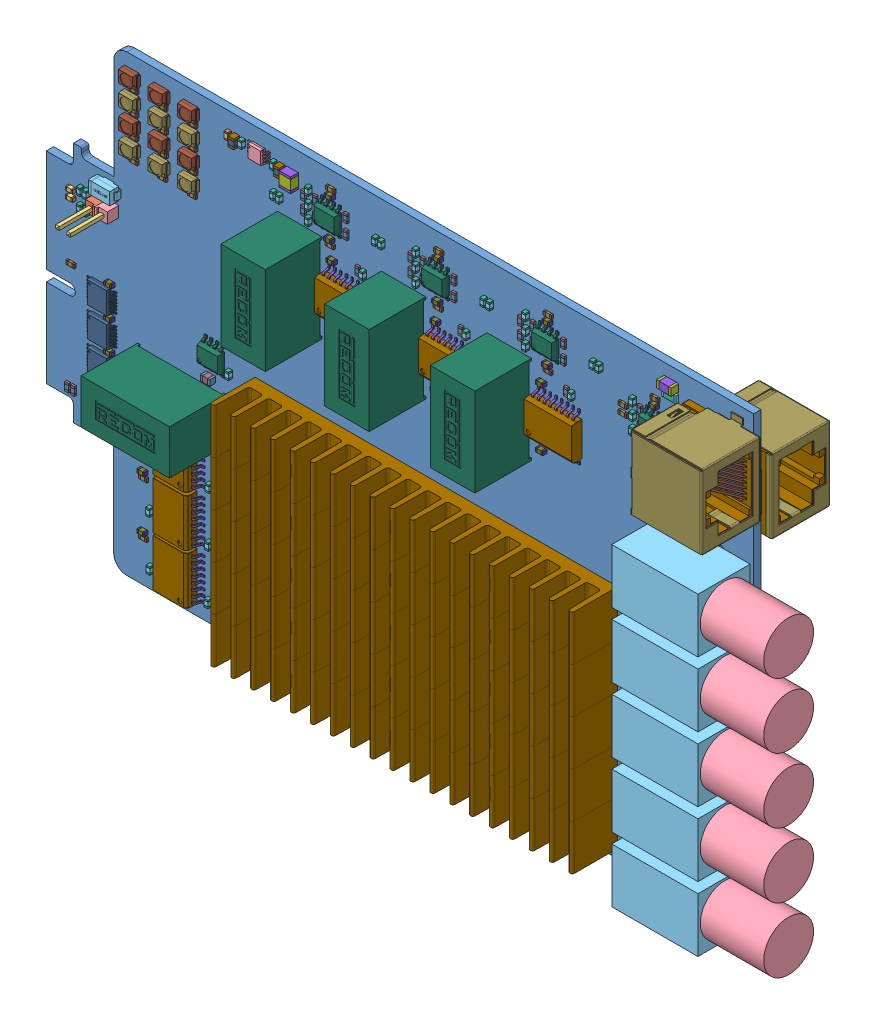
SolidWorks assembly 1166V10, configuration Standard. Lengths in mm. (continued)
Components (placement in the parent): (continued)
- 1166V10.step-1: 1166V10.step [Standard] at origin size (170.01 100 28.53) (continued)
  - R204.step-1: R204.step [Standard] at origin size (1.85 0.85 0.45) (continued)
    - 6547171152.step-1: 6547171152.step [Standard] at (32.45 80.2 0) size (0.95 0.85 0.45)
      - Extruded-6.step-1: Extruded-6.step [Standard] at origin size (0.95 0.85 0.45)
  - R202.step-1: R202.step [Standard] at origin size (1.85 0.85 0.45)
    - 6547171712.step-1: 6547171712.step [Standard] at (33.25 93.8 0) size (0.45 0.85 0.45)
      - Extruded-5.step-1: Extruded-5.step [Standard] at origin size (0.45 0.85 0.45)
    - 6547171712.step-2: 6547171712.step [Standard] at (31.85 93.8 0) size (0.45 0.85 0.45)
      - Extruded-5.step-1: Extruded-5.step [Standard] at origin size (0.45 0.85 0.45)
    - 6547171152.step-1: 6547171152.step [Standard] at (32.55 93.8 0) size (0.95 0.85 0.45)
      - Extruded-6.step-1: Extruded-6.step [Standard] at origin size (0.95 0.85 0.45)
  - R201.step-1: R201.step [Standard] at origin size (1.85 0.85 0.45)
    - 6547171712.step-1: 6547171712.step [Standard] at (33.25 89.3 0) size (0.45 0.85 0.45)
      - Extruded-5.step-1: Extruded-5.step [Standard] at origin size (0.45 0.85 0.45)
    - 6547171712.step-2: 6547171712.step [Standard] at (31.85 89.3 0) size (0.45 0.85 0.45)
      - Extruded-5.step-1: Extruded-5.step [Standard] at origin size (0.45 0.85 0.45)
    - 6547171152.step-1: 6547171152.step [Standard] at (32.55 89.3 0) size (0.95 0.85 0.45)
      - Extruded-6.step-1: Extruded-6.step [Standard] at origin size (0.95 0.85 0.45)
  - Q202.step-1: Q202.step [Standard] at origin size (12 12 1)
    - 6545154800.step-1: 6545154800.step [Standard] at (114 14.75 -2.622) size (12 12 1)
      - Extruded-13.step-1: Extruded-13.step [Standard] at origin size (12 12 1)
  - Q201.step-1: Q201.step [Standard] at origin size (12 12 1)
    - 6545154800.step-1: 6545154800.step [Standard] at (114 33.25 -2.622) size (12 12 1)
      - Extruded-13.step-1: Extruded-13.step [Standard] at origin size (12 12 1)
  - L206.step-1: L206.step [Standard] at origin size (2 1.6 1)
    - 6545385936.step-1: 6545385936.step [Standard] at (107.425 7 -2.622) size (2 1.6 1)
      - Extruded-14.step-1: Extruded-14.step [Standard] at origin size (2 1.6 1)
  - L203.step-1: L203.step [Standard] at origin size (2 1.6 1)
    - 6545385936.step-1: 6545385936.step [Standard] at (107.675 25.5 -2.622) size (2 1.6 1)
      - Extruded-14.step-1: Extruded-14.step [Standard] at origin size (2 1.6 1)
  - IC202.step-1: IC202.step [Standard] at origin size (10.5 10.6 2.6)
    - SOIC-16-300.step-1: SOIC-16-300.step [Standard] at (113.1491 76.5001 1.4) x (-1 0 0) z (0 1 0) size (10.5 2.6 10.6)
      - User_Library-SOIC-16-300_pin_SOIC_SO-300_1.step-1: User_Library-SOIC-16-300_pin_SOIC_SO-300_1.step [Standard] at (0.635 0 -3.8) x (-1 0 0) z (0 0 -1) size (0.4 1.55 1.5)
      - User_Library-SOIC-16-300_pin_SOIC_SO-300_1.step-2: User_Library-SOIC-16-300_pin_SOIC_SO-300_1.step [Standard] at (1.905 0 -3.8) x (-1 0 0) z (0 0 -1) size (0.4 1.55 1.5)
      - User_Library-SOIC-16-300_pin_SOIC_SO-300_1.step-3: User_Library-SOIC-16-300_pin_SOIC_SO-300_1.step [Standard] at (4.445 0 -3.8) x (-1 0 0) z (0 0 -1) size (0.4 1.55 1.5)
      - User_Library-SOIC-16-300_SOIC_300_SOIC_10.5X7.6_1.step-1: User_Library-SOIC-16-300_SOIC_300_SOIC_10.5X7.6_1.step [Standard] at origin size (10.5 2.35 7.6)
      - User_Library-SOIC-16-300_pin_SOIC_SO-300_1.step-4: User_Library-SOIC-16-300_pin_SOIC_SO-300_1.step [Standard] at (-3.175 0 -3.8) x (-1 0 0) z (0 0 -1) size (0.4 1.55 1.5)
      - User_Library-SOIC-16-300_pin_SOIC_SO-300_1.step-5: User_Library-SOIC-16-300_pin_SOIC_SO-300_1.step [Standard] at (-3.175 0 3.8) size (0.4 1.55 1.5)
      - User_Library-SOIC-16-300_pin_SOIC_SO-300_1.step-6: User_Library-SOIC-16-300_pin_SOIC_SO-300_1.step [Standard] at (1.905 0 3.8) size (0.4 1.55 1.5)
      - User_Library-SOIC-16-300_pin_SOIC_SO-300_1.step-7: User_Library-SOIC-16-300_pin_SOIC_SO-300_1.step [Standard] at (-1.905 0 3.8) size (0.4 1.55 1.5)
      - User_Library-SOIC-16-300_pin_SOIC_SO-300_1.step-8: User_Library-SOIC-16-300_pin_SOIC_SO-300_1.step [Standard] at (0.635 0 3.8) size (0.4 1.55 1.5)
      - User_Library-SOIC-16-300_pin_SOIC_SO-300_1.step-9: User_Library-SOIC-16-300_pin_SOIC_SO-300_1.step [Standard] at (3.175 0 3.8) size (0.4 1.55 1.5)
      - User_Library-SOIC-16-300_pin_SOIC_SO-300_1.step-10: User_Library-SOIC-16-300_pin_SOIC_SO-300_1.step [Standard] at (4.445 0 3.8) size (0.4 1.55 1.5)
      - User_Library-SOIC-16-300_pin_SOIC_SO-300_1.step-11: User_Library-SOIC-16-300_pin_SOIC_SO-300_1.step [Standard] at (-0.635 0 -3.8) x (-1 0 0) z (0 0 -1) size (0.4 1.55 1.5)
      - User_Library-SOIC-16-300_pin_SOIC_SO-300_1.step-12: User_Library-SOIC-16-300_pin_SOIC_SO-300_1.step [Standard] at (-4.445 0 3.8) size (0.4 1.55 1.5)
      - User_Library-SOIC-16-300_pin_SOIC_SO-300_1.step-13: User_Library-SOIC-16-300_pin_SOIC_SO-300_1.step [Standard] at (3.175 0 -3.8) x (-1 0 0) z (0 0 -1) size (0.4 1.55 1.5)
      - User_Library-SOIC-16-300_pin_SOIC_SO-300_1.step-14: User_Library-SOIC-16-300_pin_SOIC_SO-300_1.step [Standard] at (-0.635 0 3.8) size (0.4 1.55 1.5)
      - User_Library-SOIC-16-300_pin_SOIC_SO-300_1.step-15: User_Library-SOIC-16-300_pin_SOIC_SO-300_1.step [Standard] at (-4.445 0 -3.8) x (-1 0 0) z (0 0 -1) size (0.4 1.55 1.5)
      - User_Library-SOIC-16-300_pin_SOIC_SO-300_1.step-16: User_Library-SOIC-16-300_pin_SOIC_SO-300_1.step [Standard] at (-1.905 0 -3.8) x (-1 0 0) z (0 0 -1) size (0.4 1.55 1.5)
  - IC101.step-1: IC101.step [Standard] at origin size (6.46 5 1.2)
    - TSSOP-14.step-1: TSSOP-14.step [Standard] at (12.3449 50.9441 0) x (1 0 0) z (0 -1 0) size (6.46 1.2 5)
  - D204.step-1: D204.step [Standard] at origin size (3.49 2.8 1.55)
    - PLCC2.step-1: PLCC2.step [Standard] at (31.9999 87 0.75) x (1 0 0) z (0 0 -1) size (3.49 2.8 1.55)
  - D203.step-1: D203.step [Standard] at origin size (3.53 2.81 1.55)
    - PLCC2_rot.step-1: PLCC2_rot.step [Standard] at (32 82.5 0.75) x (1 0 0) z (0 0 -1) size (3.53 2.81 1.55)
  - D202.step-1: D202.step [Standard] at origin size (3.49 2.8 1.55)
    - PLCC2.step-1: PLCC2.step [Standard] at (31.9999 96 0.75) x (1 0 0) z (0 0 -1) size (3.49 2.8 1.55)
  - D201.step-1: D201.step [Standard] at origin size (3.53 2.81 1.55)
    - PLCC2_rot.step-1: PLCC2_rot.step [Standard] at (32 91.5 0.75) x (1 0 0) z (0 0 -1) size (3.53 2.81 1.55)
  - C227.step-1: C227.step [Standard] at origin size (2.1 1.25 1.3)
    - 6545928368.step-1: 6545928368.step [Standard] at (110.3 7.4 -2.922) size (0.5 1.25 1.3)
      - Extruded-16.step-1: Extruded-16.step [Standard] at origin size (0.5 1.25 1.3)
    - 6545928368.step-2: 6545928368.step [Standard] at (111.9 7.4 -2.922) size (0.5 1.25 1.3)
      - Extruded-16.step-1: Extruded-16.step [Standard] at origin size (0.5 1.25 1.3)
    - 6545927808.step-1: 6545927808.step [Standard] at (111.1 7.4 -2.922) size (1.1 1.25 1.3)
      - Extruded-15.step-1: Extruded-15.step [Standard] at origin size (1.1 1.25 1.3)
  - C230.step-1: C230.step [Standard] at origin size (0.82 1.6 0.9)
    - 6549602528.step-1: 6549602528.step [Standard] at (105.1 10.025 -2.522) size (0.82 0.35 0.9)
      - Extruded-0.step-1: Extruded-0.step [Standard] at origin size (0.82 0.35 0.9)
    - 6549602528.step-2: 6549602528.step [Standard] at (105.1 11.275 -2.522) size (0.82 0.35 0.9)
      - Extruded-0.step-1: Extruded-0.step [Standard] at origin size (0.82 0.35 0.9)
    - 6547668352.step-1: 6547668352.step [Standard] at (105.1 10.65 -2.522) size (0.82 0.9 0.9)
      - Extruded.step-1: Extruded.step [Standard] at origin size (0.82 0.9 0.9)
  - C226.step-1: C226.step [Standard] at origin size (1.6 0.82 0.9)
    - 6547664912.step-1: 6547664912.step [Standard] at (105.525 16.5 -2.522) size (0.35 0.82 0.9)
      - Extruded-10.step-1: Extruded-10.step [Standard] at origin size (0.35 0.82 0.9)
    - 6547664912.step-2: 6547664912.step [Standard] at (106.775 16.5 -2.522) size (0.35 0.82 0.9)
      - Extruded-10.step-1: Extruded-10.step [Standard] at origin size (0.35 0.82 0.9)
    - 6547664352.step-1: 6547664352.step [Standard] at (106.15 16.5 -2.522) size (0.9 0.82 0.9)
      - Extruded-9.step-1: Extruded-9.step [Standard] at origin size (0.9 0.82 0.9)
  - C225.step-1: C225.step [Standard] at origin size (1.25 2.1 1.3)
    - 6549603568.step-1: 6549603568.step [Standard] at (106.7 9.1 -2.922) size (1.25 0.5 1.3)
      - Extruded-3.step-1: Extruded-3.step [Standard] at origin size (1.25 0.5 1.3)
    - 6549603568.step-2: 6549603568.step [Standard] at (106.7 10.7 -2.922) size (1.25 0.5 1.3)
      - Extruded-3.step-1: Extruded-3.step [Standard] at origin size (1.25 0.5 1.3)
    - 6549603008.step-1: 6549603008.step [Standard] at (106.7 9.9 -2.922) size (1.25 1.1 1.3)
      - Extruded-4.step-1: Extruded-4.step [Standard] at origin size (1.25 1.1 1.3)
  - C212.step-1: C212.step [Standard] at origin size (2.1 1.25 1.3)
    - 6545928368.step-1: 6545928368.step [Standard] at (111.9 25.9 -2.922) size (0.5 1.25 1.3)
      - Extruded-16.step-1: Extruded-16.step [Standard] at origin size (0.5 1.25 1.3)
    - 6545928368.step-2: 6545928368.step [Standard] at (110.3 25.9 -2.922) size (0.5 1.25 1.3)
      - Extruded-16.step-1: Extruded-16.step [Standard] at origin size (0.5 1.25 1.3)
    - 6545927808.step-1: 6545927808.step [Standard] at (111.1 25.9 -2.922) size (1.1 1.25 1.3)
      - Extruded-15.step-1: Extruded-15.step [Standard] at origin size (1.1 1.25 1.3)
  - C216.step-1: C216.step [Standard] at origin size (0.82 1.6 0.9)
    - 6549602528.step-1: 6549602528.step [Standard] at (105.1 28.425 -2.522) size (0.82 0.35 0.9)
      - Extruded-0.step-1: Extruded-0.step [Standard] at origin size (0.82 0.35 0.9)
    - 6549602528.step-2: 6549602528.step [Standard] at (105.1 29.675 -2.522) size (0.82 0.35 0.9)
      - Extruded-0.step-1: Extruded-0.step [Standard] at origin size (0.82 0.35 0.9)
    - 6547668352.step-1: 6547668352.step [Standard] at (105.1 29.05 -2.522) size (0.82 0.9 0.9)
      - Extruded.step-1: Extruded.step [Standard] at origin size (0.82 0.9 0.9)
  - C211.step-1: C211.step [Standard] at origin size (1.6 0.82 0.9)
    - 6547664912.step-1: 6547664912.step [Standard] at (105.425 34.8 -2.522) size (0.35 0.82 0.9)
      - Extruded-10.step-1: Extruded-10.step [Standard] at origin size (0.35 0.82 0.9)
    - 6547664912.step-2: 6547664912.step [Standard] at (106.675 34.8 -2.522) size (0.35 0.82 0.9)
      - Extruded-10.step-1: Extruded-10.step [Standard] at origin size (0.35 0.82 0.9)
    - 6547664352.step-1: 6547664352.step [Standard] at (106.05 34.8 -2.522) size (0.9 0.82 0.9)
      - Extruded-9.step-1: Extruded-9.step [Standard] at origin size (0.9 0.82 0.9)
  - C201.step-1: C201.step [Standard] at origin size (1.25 2.1 1.3)
    - 6549603568.step-1: 6549603568.step [Standard] at (106.7 27.6 -2.922) size (1.25 0.5 1.3)
      - Extruded-3.step-1: Extruded-3.step [Standard] at origin size (1.25 0.5 1.3)
    - 6549603568.step-2: 6549603568.step [Standard] at (106.7 29.2 -2.922) size (1.25 0.5 1.3)
      - Extruded-3.step-1: Extruded-3.step [Standard] at origin size (1.25 0.5 1.3)
    - 6549603008.step-1: 6549603008.step [Standard] at (106.7 28.4 -2.922) size (1.25 1.1 1.3)
      - Extruded-4.step-1: Extruded-4.step [Standard] at origin size (1.25 1.1 1.3)
  - R415.step-1: R415.step [Standard] at origin size (3.15 6.3 0.6)
    - 6545677968.step-1: 6545677968.step [Standard] at (134.1 3.7 -2.222) size (3.15 0.6 0.6)
      - Extruded-17.step-1: Extruded-17.step [Standard] at origin size (3.15 0.6 0.6)
    - 6545677968.step-2: 6545677968.step [Standard] at (134.1 9.4 -2.222) size (3.15 0.6 0.6)
      - Extruded-17.step-1: Extruded-17.step [Standard] at origin size (3.15 0.6 0.6)
    - 6545677568.step-1: 6545677568.step [Standard] at (134.1 6.55 -2.222) size (3.15 5.1 0.6)
      - Extruded-18.step-1: Extruded-18.step [Standard] at origin size (3.15 5.1 0.6)
  - R414.step-1: R414.step [Standard] at origin size (6.3 3.15 0.6)
    - 6545676288.step-1: 6545676288.step [Standard] at (124.9 4.4 -2.222) size (0.6 3.15 0.6)
      - Extruded-19.step-1: Extruded-19.step [Standard] at origin size (0.6 3.15 0.6)
    - 6545676288.step-2: 6545676288.step [Standard] at (130.6 4.4 -2.222) size (0.6 3.15 0.6)
      - Extruded-19.step-1: Extruded-19.step [Standard] at origin size (0.6 3.15 0.6)
    - 6545675888.step-1: 6545675888.step [Standard] at (127.75 4.4 -2.222) size (5.1 3.15 0.6)
      - Extruded-20.step-1: Extruded-20.step [Standard] at origin size (5.1 3.15 0.6)
  - R315.step-1: R315.step [Standard] at origin size (3.15 6.3 0.6)
    - 6545677968.step-1: 6545677968.step [Standard] at (134.7 28.1 -2.222) size (3.15 0.6 0.6)
      - Extruded-17.step-1: Extruded-17.step [Standard] at origin size (3.15 0.6 0.6)
    - 6545677968.step-2: 6545677968.step [Standard] at (134.7 22.4 -2.222) size (3.15 0.6 0.6)
      - Extruded-17.step-1: Extruded-17.step [Standard] at origin size (3.15 0.6 0.6)
    - 6545677568.step-1: 6545677568.step [Standard] at (134.7 25.25 -2.222) size (3.15 5.1 0.6)
      - Extruded-18.step-1: Extruded-18.step [Standard] at origin size (3.15 5.1 0.6)
  - R314.step-1: R314.step [Standard] at origin size (6.3 3.15 0.6)
    - 6545676288.step-1: 6545676288.step [Standard] at (125.6 27.2 -2.222) size (0.6 3.15 0.6)
      - Extruded-19.step-1: Extruded-19.step [Standard] at origin size (0.6 3.15 0.6)
    - 6545676288.step-2: 6545676288.step [Standard] at (131.3 27.2 -2.222) size (0.6 3.15 0.6)
      - Extruded-19.step-1: Extruded-19.step [Standard] at origin size (0.6 3.15 0.6)
    - 6545675888.step-1: 6545675888.step [Standard] at (128.45 27.2 -2.222) size (5.1 3.15 0.6)
      - Extruded-20.step-1: Extruded-20.step [Standard] at origin size (5.1 3.15 0.6)
  - R215.step-1: R215.step [Standard] at origin size (3.15 6.3 0.6)
    - 6545677968.step-1: 6545677968.step [Standard] at (134.1 44 -2.222) size (3.15 0.6 0.6)
      - Extruded-17.step-1: Extruded-17.step [Standard] at origin size (3.15 0.6 0.6)
    - 6545677968.step-2: 6545677968.step [Standard] at (134.1 38.3 -2.222) size (3.15 0.6 0.6)
      - Extruded-17.step-1: Extruded-17.step [Standard] at origin size (3.15 0.6 0.6)
    - 6545677568.step-1: 6545677568.step [Standard] at (134.1 41.15 -2.222) size (3.15 5.1 0.6)
      - Extruded-18.step-1: Extruded-18.step [Standard] at origin size (3.15 5.1 0.6)
  - R214.step-1: R214.step [Standard] at origin size (6.3 3.15 0.6)
    - 6545676288.step-1: 6545676288.step [Standard] at (128.8 47.4 -2.222) size (0.6 3.15 0.6)
      - Extruded-19.step-1: Extruded-19.step [Standard] at origin size (0.6 3.15 0.6)
    - 6545676288.step-2: 6545676288.step [Standard] at (134.5 47.4 -2.222) size (0.6 3.15 0.6)
      - Extruded-19.step-1: Extruded-19.step [Standard] at origin size (0.6 3.15 0.6)
    - 6545675888.step-1: 6545675888.step [Standard] at (131.65 47.4 -2.222) size (5.1 3.15 0.6)
      - Extruded-20.step-1: Extruded-20.step [Standard] at origin size (5.1 3.15 0.6)
  - R505.step-1: R505.step [Standard] at origin size (6.3 3.15 0.6)
    - 6545676288.step-1: 6545676288.step [Standard] at (50.7 56.5 -2.222) size (0.6 3.15 0.6)
      - Extruded-19.step-1: Extruded-19.step [Standard] at origin size (0.6 3.15 0.6)
    - 6545676288.step-2: 6545676288.step [Standard] at (56.4 56.5 -2.222) size (0.6 3.15 0.6)
      - Extruded-19.step-1: Extruded-19.step [Standard] at origin size (0.6 3.15 0.6)
    - 6545675888.step-1: 6545675888.step [Standard] at (53.55 56.5 -2.222) size (5.1 3.15 0.6)
      - Extruded-20.step-1: Extruded-20.step [Standard] at origin size (5.1 3.15 0.6)
  - R504.step-1: R504.step [Standard] at origin size (6.3 3.15 0.6)
    - 6545676288.step-1: 6545676288.step [Standard] at (44.4 60.3 -2.222) size (0.6 3.15 0.6)
      - Extruded-19.step-1: Extruded-19.step [Standard] at origin size (0.6 3.15 0.6)
    - 6545676288.step-2: 6545676288.step [Standard] at (50.1 60.3 -2.222) size (0.6 3.15 0.6)
      - Extruded-19.step-1: Extruded-19.step [Standard] at origin size (0.6 3.15 0.6)
    - 6545675888.step-1: 6545675888.step [Standard] at (47.25 60.3 -2.222) size (5.1 3.15 0.6)
      - Extruded-20.step-1: Extruded-20.step [Standard] at origin size (5.1 3.15 0.6)
  - R508.step-1: R508.step [Standard] at origin size (1.85 0.85 0.45)
    - 6547171152.step-1: 6547171152.step [Standard] at (43.95 65.3 -2.072) size (0.95 0.85 0.45)
      - Extruded-6.step-1: Extruded-6.step [Standard] at origin size (0.95 0.85 0.45)
    - 6547171712.step-1: 6547171712.step [Standard] at (43.25 65.3 -2.072) size (0.45 0.85 0.45)
      - Extruded-5.step-1: Extruded-5.step [Standard] at origin size (0.45 0.85 0.45)
    - 6547171712.step-2: 6547171712.step [Standard] at (44.65 65.3 -2.072) size (0.45 0.85 0.45)
      - Extruded-5.step-1: Extruded-5.step [Standard] at origin size (0.45 0.85 0.45)
  - R506.step-1: R506.step [Standard] at origin size (3.05 6.35 0.83)
    - CSS2H-2512.step-1: CSS2H-2512.step [Standard] at (131.8499 60.1249 -1.622) x (0 1 0) z (-1 0 0) size (6.35 0.83 3.05)
      - 3DMODEL-TEXT_ASM_2_ASM.step-1: 3DMODEL-TEXT_ASM_2_ASM.step [Standard] at origin size (6.35 0.83 3.05)
        - COPPER25__2_ASM.step-1: COPPER25__2_ASM.step [Standard] at origin size (6.35 0.77 3.05)
          - MANIFOLD_SOLID_BREP_547.step-1: MANIFOLD_SOLID_BREP_547.step [Standard] at origin size (1.68 0.77 3.05)
          - MANIFOLD_SOLID_BREP_1090.step-1: MANIFOLD_SOLID_BREP_1090.step [Standard] at origin size (1.68 0.77 3.05)
          - Open CASCADE STEP translator 6.8 1.242.1.1.1.3.step-1: Open CASCADE STEP translator 6.8 1.242.1.1.1.3.step [Standard] at origin
        - RESIST2512_3.step-1: RESIST2512_3.step [Standard] at (1.675 0.3481 0) x (1 0 0) z (0 1 0) size (3 3.05 0.48)
  - R503.step-1: R503.step [Standard] at origin size (1.85 0.85 0.45)
    - 6547171712.step-1: 6547171712.step [Standard] at (126.75 64.3 -2.072) size (0.45 0.85 0.45)
      - Extruded-5.step-1: Extruded-5.step [Standard] at origin size (0.45 0.85 0.45)
    - 6547171712.step-2: 6547171712.step [Standard] at (125.35 64.3 -2.072) size (0.45 0.85 0.45)
      - Extruded-5.step-1: Extruded-5.step [Standard] at origin size (0.45 0.85 0.45)
    - 6547171152.step-1: 6547171152.step [Standard] at (126.05 64.3 -2.072) size (0.95 0.85 0.45)
      - Extruded-6.step-1: Extruded-6.step [Standard] at origin size (0.95 0.85 0.45)
  - R502.step-1: R502.step [Standard] at origin size (1.85 0.85 0.45)
    - 6547171712.step-1: 6547171712.step [Standard] at (127.55 63 -2.072) size (0.45 0.85 0.45)
      - Extruded-5.step-1: Extruded-5.step [Standard] at origin size (0.45 0.85 0.45)
    - 6547171712.step-2: 6547171712.step [Standard] at (126.15 63 -2.072) size (0.45 0.85 0.45)
      - Extruded-5.step-1: Extruded-5.step [Standard] at origin size (0.45 0.85 0.45)
    - 6547171152.step-1: 6547171152.step [Standard] at (126.85 63 -2.072) size (0.95 0.85 0.45)
      - Extruded-6.step-1: Extruded-6.step [Standard] at origin size (0.95 0.85 0.45)
  - R501.step-1: R501.step [Standard] at origin size (1.85 0.85 0.45)
    - 6547171712.step-1: 6547171712.step [Standard] at (130.75 85.5 -2.072) size (0.45 0.85 0.45)
      - Extruded-5.step-1: Extruded-5.step [Standard] at origin size (0.45 0.85 0.45)
    - 6547171712.step-2: 6547171712.step [Standard] at (129.35 85.5 -2.072) size (0.45 0.85 0.45)
      - Extruded-5.step-1: Extruded-5.step [Standard] at origin size (0.45 0.85 0.45)
    - 6547171152.step-1: 6547171152.step [Standard] at (130.05 85.5 -2.072) size (0.95 0.85 0.45)
      - Extruded-6.step-1: Extruded-6.step [Standard] at origin size (0.95 0.85 0.45)
  - J502.step-1: J502.step [Standard] at origin size (33 12 11.5)
    - 6544611488.step-1: 6544611488.step [Standard] at (170 51.4434 6.3) x (0 -1 0) z (-1 0 0) size (11 11 14)
      - Cylinder.step-1: Cylinder.step [Standard] at origin size (11 11 14)
    - 6544611248.step-1: 6544611248.step [Standard] at (146.5 51.4 0.8) size (19 12 11.5)
      - Extruded-21.step-1: Extruded-21.step [Standard] at origin size (19 12 11.5)
  - J501.step-1: J501.step [Standard] at origin size (33 12 11.5)
    - 6544611488.step-1: 6544611488.step [Standard] at (170 65.7434 6.3) x (0 -1 0) z (-1 0 0) size (11 11 14)
      - Cylinder.step-1: Cylinder.step [Standard] at origin size (11 11 14)
    - 6544611248.step-1: 6544611248.step [Standard] at (146.5 65.7 0.8) size (19 12 11.5)
      - Extruded-21.step-1: Extruded-21.step [Standard] at origin size (19 12 11.5)
  - IC502.step-1: IC502.step [Standard] at origin size (4.83 10.64 1.7)
    - SOIC-8_Wide.step-1: SOIC-8_Wide.step [Standard] at (46.0701 76.3999 -1.622) x (1 0 0) z (0 1 0) size (4.83 1.7 10.64)
  - IC501.step-1: IC501.step [Standard] at origin size (10.5 10.6 2.6)
    - SOIC-16-300.step-1: SOIC-16-300.step [Standard] at (128.4509 76.5501 -3.022) x (1 0 0) z (0 1 0) size (10.5 2.6 10.6)
      - User_Library-SOIC-16-300_pin_SOIC_SO-300_1.step-1: User_Library-SOIC-16-300_pin_SOIC_SO-300_1.step [Standard] at (0.635 0 -3.8) x (-1 0 0) z (0 0 -1) size (0.4 1.55 1.5)
      - User_Library-SOIC-16-300_pin_SOIC_SO-300_1.step-2: User_Library-SOIC-16-300_pin_SOIC_SO-300_1.step [Standard] at (1.905 0 -3.8) x (-1 0 0) z (0 0 -1) size (0.4 1.55 1.5)
      - User_Library-SOIC-16-300_pin_SOIC_SO-300_1.step-3: User_Library-SOIC-16-300_pin_SOIC_SO-300_1.step [Standard] at (4.445 0 -3.8) x (-1 0 0) z (0 0 -1) size (0.4 1.55 1.5)
      - User_Library-SOIC-16-300_SOIC_300_SOIC_10.5X7.6_1.step-1: User_Library-SOIC-16-300_SOIC_300_SOIC_10.5X7.6_1.step [Standard] at origin size (10.5 2.35 7.6)
      - User_Library-SOIC-16-300_pin_SOIC_SO-300_1.step-4: User_Library-SOIC-16-300_pin_SOIC_SO-300_1.step [Standard] at (-3.175 0 -3.8) x (-1 0 0) z (0 0 -1) size (0.4 1.55 1.5)
      - User_Library-SOIC-16-300_pin_SOIC_SO-300_1.step-5: User_Library-SOIC-16-300_pin_SOIC_SO-300_1.step [Standard] at (-3.175 0 3.8) size (0.4 1.55 1.5)
      - User_Library-SOIC-16-300_pin_SOIC_SO-300_1.step-6: User_Library-SOIC-16-300_pin_SOIC_SO-300_1.step [Standard] at (1.905 0 3.8) size (0.4 1.55 1.5)
      - User_Library-SOIC-16-300_pin_SOIC_SO-300_1.step-7: User_Library-SOIC-16-300_pin_SOIC_SO-300_1.step [Standard] at (-1.905 0 3.8) size (0.4 1.55 1.5)
      - User_Library-SOIC-16-300_pin_SOIC_SO-300_1.step-8: User_Library-SOIC-16-300_pin_SOIC_SO-300_1.step [Standard] at (0.635 0 3.8) size (0.4 1.55 1.5)
      - User_Library-SOIC-16-300_pin_SOIC_SO-300_1.step-9: User_Library-SOIC-16-300_pin_SOIC_SO-300_1.step [Standard] at (3.175 0 3.8) size (0.4 1.55 1.5)
      - User_Library-SOIC-16-300_pin_SOIC_SO-300_1.step-10: User_Library-SOIC-16-300_pin_SOIC_SO-300_1.step [Standard] at (4.445 0 3.8) size (0.4 1.55 1.5)
      - User_Library-SOIC-16-300_pin_SOIC_SO-300_1.step-11: User_Library-SOIC-16-300_pin_SOIC_SO-300_1.step [Standard] at (-0.635 0 -3.8) x (-1 0 0) z (0 0 -1) size (0.4 1.55 1.5)
      - User_Library-SOIC-16-300_pin_SOIC_SO-300_1.step-12: User_Library-SOIC-16-300_pin_SOIC_SO-300_1.step [Standard] at (-4.445 0 3.8) size (0.4 1.55 1.5)
      - User_Library-SOIC-16-300_pin_SOIC_SO-300_1.step-13: User_Library-SOIC-16-300_pin_SOIC_SO-300_1.step [Standard] at (3.175 0 -3.8) x (-1 0 0) z (0 0 -1) size (0.4 1.55 1.5)
      - User_Library-SOIC-16-300_pin_SOIC_SO-300_1.step-14: User_Library-SOIC-16-300_pin_SOIC_SO-300_1.step [Standard] at (-0.635 0 3.8) size (0.4 1.55 1.5)
      - User_Library-SOIC-16-300_pin_SOIC_SO-300_1.step-15: User_Library-SOIC-16-300_pin_SOIC_SO-300_1.step [Standard] at (-4.445 0 -3.8) x (-1 0 0) z (0 0 -1) size (0.4 1.55 1.5)
      - User_Library-SOIC-16-300_pin_SOIC_SO-300_1.step-16: User_Library-SOIC-16-300_pin_SOIC_SO-300_1.step [Standard] at (-1.905 0 -3.8) x (-1 0 0) z (0 0 -1) size (0.4 1.55 1.5)
  - CF504.step-1: CF504.step [Standard] at origin size (1.6 0.82 0.9)
    - 6547664912.step-1: 6547664912.step [Standard] at (45.475 67.9 -2.522) size (0.35 0.82 0.9)
      - Extruded-10.step-1: Extruded-10.step [Standard] at origin size (0.35 0.82 0.9)
    - 6547664912.step-2: 6547664912.step [Standard] at (44.225 67.9 -2.522) size (0.35 0.82 0.9)
      - Extruded-10.step-1: Extruded-10.step [Standard] at origin size (0.35 0.82 0.9)
    - 6547664352.step-1: 6547664352.step [Standard] at (44.85 67.9 -2.522) size (0.9 0.82 0.9)
      - Extruded-9.step-1: Extruded-9.step [Standard] at origin size (0.9 0.82 0.9)
  - CF503.step-1: CF503.step [Standard] at origin size (1.6 0.82 0.9)
    - 6547664912.step-1: 6547664912.step [Standard] at (45.475 69.2 -2.522) size (0.35 0.82 0.9)
      - Extruded-10.step-1: Extruded-10.step [Standard] at origin size (0.35 0.82 0.9)
    - 6547664912.step-2: 6547664912.step [Standard] at (44.225 69.2 -2.522) size (0.35 0.82 0.9)
      - Extruded-10.step-1: Extruded-10.step [Standard] at origin size (0.35 0.82 0.9)
    - 6547664352.step-1: 6547664352.step [Standard] at (44.85 69.2 -2.522) size (0.9 0.82 0.9)
      - Extruded-9.step-1: Extruded-9.step [Standard] at origin size (0.9 0.82 0.9)
  - CF502.step-1: CF502.step [Standard] at origin size (1.6 0.82 0.9)
    - 6547664912.step-1: 6547664912.step [Standard] at (47.625 81.8 -2.522) size (0.35 0.82 0.9)
      - Extruded-10.step-1: Extruded-10.step [Standard] at origin size (0.35 0.82 0.9)
    - 6547664912.step-2: 6547664912.step [Standard] at (48.875 81.8 -2.522) size (0.35 0.82 0.9)
      - Extruded-10.step-1: Extruded-10.step [Standard] at origin size (0.35 0.82 0.9)
    - 6547664352.step-1: 6547664352.step [Standard] at (48.25 81.8 -2.522) size (0.9 0.82 0.9)
      - Extruded-9.step-1: Extruded-9.step [Standard] at origin size (0.9 0.82 0.9)
  - CF501.step-1: CF501.step [Standard] at origin size (1.6 0.82 0.9)
    - 6547664912.step-1: 6547664912.step [Standard] at (47.625 83.1 -2.522) size (0.35 0.82 0.9)
      - Extruded-10.step-1: Extruded-10.step [Standard] at origin size (0.35 0.82 0.9)
    - 6547664912.step-2: 6547664912.step [Standard] at (48.875 83.1 -2.522) size (0.35 0.82 0.9)
      - Extruded-10.step-1: Extruded-10.step [Standard] at origin size (0.35 0.82 0.9)
    - 6547664352.step-1: 6547664352.step [Standard] at (48.25 83.1 -2.522) size (0.9 0.82 0.9)
      - Extruded-9.step-1: Extruded-9.step [Standard] at origin size (0.9 0.82 0.9)
  - C515.step-1: C515.step [Standard] at origin size (5 5.7 2.5)
    - 6545679008.step-1: 6545679008.step [Standard] at (100.4 56.575 -4.122) size (5 0.65 2.5)
      - Extruded-11.step-1: Extruded-11.step [Standard] at origin size (5 0.65 2.5)
    - 6545679008.step-2: 6545679008.step [Standard] at (100.4 51.525 -4.122) size (5 0.65 2.5)
      - Extruded-11.step-1: Extruded-11.step [Standard] at origin size (5 0.65 2.5)
    - 6545678448.step-1: 6545678448.step [Standard] at (100.4 54.05 -4.122) size (5 4.4 2.5)
      - Extruded-12.step-1: Extruded-12.step [Standard] at origin size (5 4.4 2.5)
  - C514.step-1: C514.step [Standard] at origin size (5 5.7 2.5)
    - 6545679008.step-1: 6545679008.step [Standard] at (73.6 56.775 -4.122) size (5 0.65 2.5)
      - Extruded-11.step-1: Extruded-11.step [Standard] at origin size (5 0.65 2.5)
    - 6545679008.step-2: 6545679008.step [Standard] at (73.6 51.725 -4.122) size (5 0.65 2.5)
      - Extruded-11.step-1: Extruded-11.step [Standard] at origin size (5 0.65 2.5)
    - 6545678448.step-1: 6545678448.step [Standard] at (73.6 54.25 -4.122) size (5 4.4 2.5)
      - Extruded-12.step-1: Extruded-12.step [Standard] at origin size (5 4.4 2.5)
  - C513.step-1: C513.step [Standard] at origin size (5 5.7 2.5)
    - 6545679008.step-1: 6545679008.step [Standard] at (127.3 57.375 -4.122) size (5 0.65 2.5)
      - Extruded-11.step-1: Extruded-11.step [Standard] at origin size (5 0.65 2.5)
    - 6545679008.step-2: 6545679008.step [Standard] at (127.3 52.325 -4.122) size (5 0.65 2.5)
      - Extruded-11.step-1: Extruded-11.step [Standard] at origin size (5 0.65 2.5)
    - 6545678448.step-1: 6545678448.step [Standard] at (127.3 54.85 -4.122) size (5 4.4 2.5)
      - Extruded-12.step-1: Extruded-12.step [Standard] at origin size (5 4.4 2.5)
  - C511.step-1: C511.step [Standard] at origin size (1.6 0.82 0.9)
    - 6547664912.step-1: 6547664912.step [Standard] at (43.325 66.6 -2.522) size (0.35 0.82 0.9)
      - Extruded-10.step-1: Extruded-10.step [Standard] at origin size (0.35 0.82 0.9)
    - 6547664912.step-2: 6547664912.step [Standard] at (44.575 66.6 -2.522) size (0.35 0.82 0.9)
      - Extruded-10.step-1: Extruded-10.step [Standard] at origin size (0.35 0.82 0.9)
    - 6547664352.step-1: 6547664352.step [Standard] at (43.95 66.6 -2.522) size (0.9 0.82 0.9)
      - Extruded-9.step-1: Extruded-9.step [Standard] at origin size (0.9 0.82 0.9)
  - C509.step-1: C509.step [Standard] at origin size (1.6 0.82 0.9)
    - 6547664352.step-1: 6547664352.step [Standard] at (126.05 65.7 -2.522) size (0.9 0.82 0.9)
      - Extruded-9.step-1: Extruded-9.step [Standard] at origin size (0.9 0.82 0.9)
    - 6547664912.step-1: 6547664912.step [Standard] at (126.675 65.7 -2.522) size (0.35 0.82 0.9)
      - Extruded-10.step-1: Extruded-10.step [Standard] at origin size (0.35 0.82 0.9)
    - 6547664912.step-2: 6547664912.step [Standard] at (125.425 65.7 -2.522) size (0.35 0.82 0.9)
      - Extruded-10.step-1: Extruded-10.step [Standard] at origin size (0.35 0.82 0.9)
  - C508.step-1: C508.step [Standard] at origin size (3.2 1.6 1.7)
    - 6547444720.step-1: 6547444720.step [Standard] at (127.3 67.5 -3.322) size (0.5 1.6 1.7)
      - Extruded-22.step-1: Extruded-22.step [Standard] at origin size (0.5 1.6 1.7)
    - 6547444720.step-2: 6547444720.step [Standard] at (124.6 67.5 -3.322) size (0.5 1.6 1.7)
      - Extruded-22.step-1: Extruded-22.step [Standard] at origin size (0.5 1.6 1.7)
    - 6547445040.step-1: 6547445040.step [Standard] at (125.95 67.5 -3.322) size (2.2 1.6 1.7)
      - Extruded-23.step-1: Extruded-23.step [Standard] at origin size (2.2 1.6 1.7)
  - C507.step-1: C507.step [Standard] at origin size (3.2 1.6 1.7)
    - 6547444720.step-1: 6547444720.step [Standard] at (127.3 69.6 -3.322) size (0.5 1.6 1.7)
      - Extruded-22.step-1: Extruded-22.step [Standard] at origin size (0.5 1.6 1.7)
    - 6547444720.step-2: 6547444720.step [Standard] at (124.6 69.6 -3.322) size (0.5 1.6 1.7)
      - Extruded-22.step-1: Extruded-22.step [Standard] at origin size (0.5 1.6 1.7)
    - 6547445040.step-1: 6547445040.step [Standard] at (125.95 69.6 -3.322) size (2.2 1.6 1.7)
      - Extruded-23.step-1: Extruded-23.step [Standard] at origin size (2.2 1.6 1.7)
  - C506.step-1: C506.step [Standard] at origin size (1.6 0.82 0.9)
    - 6547664352.step-1: 6547664352.step [Standard] at (132.75 68.8 -2.522) size (0.9 0.82 0.9)
      - Extruded-9.step-1: Extruded-9.step [Standard] at origin size (0.9 0.82 0.9)
    - 6547664912.step-1: 6547664912.step [Standard] at (132.125 68.8 -2.522) size (0.35 0.82 0.9)
      - Extruded-10.step-1: Extruded-10.step [Standard] at origin size (0.35 0.82 0.9)
    - 6547664912.step-2: 6547664912.step [Standard] at (133.375 68.8 -2.522) size (0.35 0.82 0.9)
      - Extruded-10.step-1: Extruded-10.step [Standard] at origin size (0.35 0.82 0.9)
  - C505.step-1: C505.step [Standard] at origin size (1.6 0.82 0.9)
    - 6547664352.step-1: 6547664352.step [Standard] at (132.75 70 -2.522) size (0.9 0.82 0.9)
      - Extruded-9.step-1: Extruded-9.step [Standard] at origin size (0.9 0.82 0.9)
    - 6547664912.step-1: 6547664912.step [Standard] at (132.125 70 -2.522) size (0.35 0.82 0.9)
      - Extruded-10.step-1: Extruded-10.step [Standard] at origin size (0.35 0.82 0.9)
    - 6547664912.step-2: 6547664912.step [Standard] at (133.375 70 -2.522) size (0.35 0.82 0.9)
      - Extruded-10.step-1: Extruded-10.step [Standard] at origin size (0.35 0.82 0.9)
  - C504.step-1: C504.step [Standard] at origin size (1.6 0.82 0.9)
    - 6547664352.step-1: 6547664352.step [Standard] at (129.85 70 -2.522) size (0.9 0.82 0.9)
      - Extruded-9.step-1: Extruded-9.step [Standard] at origin size (0.9 0.82 0.9)
    - 6547664912.step-1: 6547664912.step [Standard] at (130.475 70 -2.522) size (0.35 0.82 0.9)
      - Extruded-10.step-1: Extruded-10.step [Standard] at origin size (0.35 0.82 0.9)
    - 6547664912.step-2: 6547664912.step [Standard] at (129.225 70 -2.522) size (0.35 0.82 0.9)
      - Extruded-10.step-1: Extruded-10.step [Standard] at origin size (0.35 0.82 0.9)
  - C503.step-1: C503.step [Standard] at origin size (3.2 1.6 1.7)
    - 6547444720.step-1: 6547444720.step [Standard] at (127.4 83.4 -3.322) size (0.5 1.6 1.7)
      - Extruded-22.step-1: Extruded-22.step [Standard] at origin size (0.5 1.6 1.7)
    - 6547444720.step-2: 6547444720.step [Standard] at (124.7 83.4 -3.322) size (0.5 1.6 1.7)
      - Extruded-22.step-1: Extruded-22.step [Standard] at origin size (0.5 1.6 1.7)
    - 6547445040.step-1: 6547445040.step [Standard] at (126.05 83.4 -3.322) size (2.2 1.6 1.7)
      - Extruded-23.step-1: Extruded-23.step [Standard] at origin size (2.2 1.6 1.7)
  - C502.step-1: C502.step [Standard] at origin size (3.2 1.6 1.7)
    - 6547444720.step-1: 6547444720.step [Standard] at (127.4 85.5 -3.322) size (0.5 1.6 1.7)
      - Extruded-22.step-1: Extruded-22.step [Standard] at origin size (0.5 1.6 1.7)
    - 6547444720.step-2: 6547444720.step [Standard] at (124.7 85.5 -3.322) size (0.5 1.6 1.7)
      - Extruded-22.step-1: Extruded-22.step [Standard] at origin size (0.5 1.6 1.7)
    - 6547445040.step-1: 6547445040.step [Standard] at (126.05 85.5 -3.322) size (2.2 1.6 1.7)
      - Extruded-23.step-1: Extruded-23.step [Standard] at origin size (2.2 1.6 1.7)
  - C501.step-1: C501.step [Standard] at origin size (1.6 0.82 0.9)
    - 6547664352.step-1: 6547664352.step [Standard] at (132.05 83 -2.522) size (0.9 0.82 0.9)
      - Extruded-9.step-1: Extruded-9.step [Standard] at origin size (0.9 0.82 0.9)
    - 6547664912.step-1: 6547664912.step [Standard] at (132.675 83 -2.522) size (0.35 0.82 0.9)
      - Extruded-10.step-1: Extruded-10.step [Standard] at origin size (0.35 0.82 0.9)
    - 6547664912.step-2: 6547664912.step [Standard] at (131.425 83 -2.522) size (0.35 0.82 0.9)
      - Extruded-10.step-1: Extruded-10.step [Standard] at origin size (0.35 0.82 0.9)
  - R410.step-1: R410.step [Standard] at origin size (6.35 3.05 0.83)
    - CSS2H-2512.step-1: CSS2H-2512.step [Standard] at (128.3249 14.3501 -1.622) x (1 0 0) z (0 1 0) size (6.35 0.83 3.05)
      - 3DMODEL-TEXT_ASM_2_ASM.step-1: 3DMODEL-TEXT_ASM_2_ASM.step [Standard] at origin size (6.35 0.83 3.05)
        - COPPER25__2_ASM.step-1: COPPER25__2_ASM.step [Standard] at origin size (6.35 0.77 3.05)
          - MANIFOLD_SOLID_BREP_547.step-1: MANIFOLD_SOLID_BREP_547.step [Standard] at origin size (1.68 0.77 3.05)
          - MANIFOLD_SOLID_BREP_1090.step-1: MANIFOLD_SOLID_BREP_1090.step [Standard] at origin size (1.68 0.77 3.05)
          - Open CASCADE STEP translator 6.8 1.242.1.1.1.3.step-1: Open CASCADE STEP translator 6.8 1.242.1.1.1.3.step [Standard] at origin
        - RESIST2512_3.step-1: RESIST2512_3.step [Standard] at (1.675 0.3481 0) x (1 0 0) z (0 1 0) size (3 3.05 0.48)
  - R409.step-1: R409.step [Standard] at origin size (0.85 1.85 0.45)
    - 6549605008.step-1: 6549605008.step [Standard] at (63.6 63.05 -2.072) size (0.85 0.45 0.45)
      - Extruded-7.step-1: Extruded-7.step [Standard] at origin size (0.85 0.45 0.45)
    - 6549605008.step-2: 6549605008.step [Standard] at (63.6 64.45 -2.072) size (0.85 0.45 0.45)
      - Extruded-7.step-1: Extruded-7.step [Standard] at origin size (0.85 0.45 0.45)
    - 6549605488.step-1: 6549605488.step [Standard] at (63.6 63.75 -2.072) size (0.85 0.95 0.45)
      - Extruded-8.step-1: Extruded-8.step [Standard] at origin size (0.85 0.95 0.45)
  - R408.step-1: R408.step [Standard] at origin size (0.85 1.85 0.45)
    - 6549605008.step-1: 6549605008.step [Standard] at (64.9 63.05 -2.072) size (0.85 0.45 0.45)
      - Extruded-7.step-1: Extruded-7.step [Standard] at origin size (0.85 0.45 0.45)
    - 6549605008.step-2: 6549605008.step [Standard] at (64.9 64.45 -2.072) size (0.85 0.45 0.45)
      - Extruded-7.step-1: Extruded-7.step [Standard] at origin size (0.85 0.45 0.45)
    - 6549605488.step-1: 6549605488.step [Standard] at (64.9 63.75 -2.072) size (0.85 0.95 0.45)
      - Extruded-8.step-1: Extruded-8.step [Standard] at origin size (0.85 0.95 0.45)
  - R403.step-1: R403.step [Standard] at origin size (1.85 0.85 0.45)
    - 6547171712.step-1: 6547171712.step [Standard] at (69.05 85.5 -2.072) size (0.45 0.85 0.45)
      - Extruded-5.step-1: Extruded-5.step [Standard] at origin size (0.45 0.85 0.45)
    - 6547171712.step-2: 6547171712.step [Standard] at (67.65 85.5 -2.072) size (0.45 0.85 0.45)
      - Extruded-5.step-1: Extruded-5.step [Standard] at origin size (0.45 0.85 0.45)
    - 6547171152.step-1: 6547171152.step [Standard] at (68.35 85.5 -2.072) size (0.95 0.85 0.45)
      - Extruded-6.step-1: Extruded-6.step [Standard] at origin size (0.95 0.85 0.45)
  - R310.step-1: R310.step [Standard] at origin size (6.35 3.05 0.83)
    - CSS2H-2512.step-1: CSS2H-2512.step [Standard] at (128.3249 20.4501 -1.622) x (1 0 0) z (0 1 0) size (6.35 0.83 3.05)
      - 3DMODEL-TEXT_ASM_2_ASM.step-1: 3DMODEL-TEXT_ASM_2_ASM.step [Standard] at origin size (6.35 0.83 3.05)
        - COPPER25__2_ASM.step-1: COPPER25__2_ASM.step [Standard] at origin size (6.35 0.77 3.05)
          - MANIFOLD_SOLID_BREP_547.step-1: MANIFOLD_SOLID_BREP_547.step [Standard] at origin size (1.68 0.77 3.05)
          - MANIFOLD_SOLID_BREP_1090.step-1: MANIFOLD_SOLID_BREP_1090.step [Standard] at origin size (1.68 0.77 3.05)
          - Open CASCADE STEP translator 6.8 1.242.1.1.1.3.step-1: Open CASCADE STEP translator 6.8 1.242.1.1.1.3.step [Standard] at origin
        - RESIST2512_3.step-1: RESIST2512_3.step [Standard] at (1.675 0.3481 0) x (1 0 0) z (0 1 0) size (3 3.05 0.48)
  - R309.step-1: R309.step [Standard] at origin size (0.85 1.85 0.45)
    - 6549605008.step-1: 6549605008.step [Standard] at (86.5 62.75 -2.072) size (0.85 0.45 0.45)
      - Extruded-7.step-1: Extruded-7.step [Standard] at origin size (0.85 0.45 0.45)
    - 6549605008.step-2: 6549605008.step [Standard] at (86.5 64.15 -2.072) size (0.85 0.45 0.45)
      - Extruded-7.step-1: Extruded-7.step [Standard] at origin size (0.85 0.45 0.45)
    - 6549605488.step-1: 6549605488.step [Standard] at (86.5 63.45 -2.072) size (0.85 0.95 0.45)
      - Extruded-8.step-1: Extruded-8.step [Standard] at origin size (0.85 0.95 0.45)
  - R308.step-1: R308.step [Standard] at origin size (0.85 1.85 0.45)
    - 6549605008.step-1: 6549605008.step [Standard] at (87.8 62.75 -2.072) size (0.85 0.45 0.45)
      - Extruded-7.step-1: Extruded-7.step [Standard] at origin size (0.85 0.45 0.45)
    - 6549605008.step-2: 6549605008.step [Standard] at (87.8 64.15 -2.072) size (0.85 0.45 0.45)
      - Extruded-7.step-1: Extruded-7.step [Standard] at origin size (0.85 0.45 0.45)
    - 6549605488.step-1: 6549605488.step [Standard] at (87.8 63.45 -2.072) size (0.85 0.95 0.45)
      - Extruded-8.step-1: Extruded-8.step [Standard] at origin size (0.85 0.95 0.45)
  - R303.step-1: R303.step [Standard] at origin size (1.85 0.85 0.45)
    - 6547171712.step-1: 6547171712.step [Standard] at (91.95 85.5 -2.072) size (0.45 0.85 0.45)
      - Extruded-5.step-1: Extruded-5.step [Standard] at origin size (0.45 0.85 0.45)
    - 6547171712.step-2: 6547171712.step [Standard] at (90.55 85.5 -2.072) size (0.45 0.85 0.45)
      - Extruded-5.step-1: Extruded-5.step [Standard] at origin size (0.45 0.85 0.45)
    - 6547171152.step-1: 6547171152.step [Standard] at (91.25 85.5 -2.072) size (0.95 0.85 0.45)
      - Extruded-6.step-1: Extruded-6.step [Standard] at origin size (0.95 0.85 0.45)
  - R210.step-1: R210.step [Standard] at origin size (6.35 3.05 0.83)
    - CSS2H-2512.step-1: CSS2H-2512.step [Standard] at (128.3249 36.4501 -1.622) x (1 0 0) z (0 1 0) size (6.35 0.83 3.05)
      - 3DMODEL-TEXT_ASM_2_ASM.step-1: 3DMODEL-TEXT_ASM_2_ASM.step [Standard] at origin size (6.35 0.83 3.05)
        - COPPER25__2_ASM.step-1: COPPER25__2_ASM.step [Standard] at origin size (6.35 0.77 3.05)
          - MANIFOLD_SOLID_BREP_547.step-1: MANIFOLD_SOLID_BREP_547.step [Standard] at origin size (1.68 0.77 3.05)
          - MANIFOLD_SOLID_BREP_1090.step-1: MANIFOLD_SOLID_BREP_1090.step [Standard] at origin size (1.68 0.77 3.05)
          - Open CASCADE STEP translator 6.8 1.242.1.1.1.3.step-1: Open CASCADE STEP translator 6.8 1.242.1.1.1.3.step [Standard] at origin
        - RESIST2512_3.step-1: RESIST2512_3.step [Standard] at (1.675 0.3481 0) x (1 0 0) z (0 1 0) size (3 3.05 0.48)
  - R203.step-1: R203.step [Standard] at origin size (1.85 0.85 0.45)
    - 6547171712.step-1: 6547171712.step [Standard] at (115.15 85.5 -2.072) size (0.45 0.85 0.45)
      - Extruded-5.step-1: Extruded-5.step [Standard] at origin size (0.45 0.85 0.45)
    - 6547171712.step-2: 6547171712.step [Standard] at (113.75 85.5 -2.072) size (0.45 0.85 0.45)
      - Extruded-5.step-1: Extruded-5.step [Standard] at origin size (0.45 0.85 0.45)
    - 6547171152.step-1: 6547171152.step [Standard] at (114.45 85.5 -2.072) size (0.95 0.85 0.45)
      - Extruded-6.step-1: Extruded-6.step [Standard] at origin size (0.95 0.85 0.45)
  - R208.step-1: R208.step [Standard] at origin size (0.85 1.85 0.45)
    - 6549605008.step-1: 6549605008.step [Standard] at (111.3 62.85 -2.072) size (0.85 0.45 0.45)
      - Extruded-7.step-1: Extruded-7.step [Standard] at origin size (0.85 0.45 0.45)
    - 6549605008.step-2: 6549605008.step [Standard] at (111.3 64.25 -2.072) size (0.85 0.45 0.45)
      - Extruded-7.step-1: Extruded-7.step [Standard] at origin size (0.85 0.45 0.45)
    - 6549605488.step-1: 6549605488.step [Standard] at (111.3 63.55 -2.072) size (0.85 0.95 0.45)
      - Extruded-8.step-1: Extruded-8.step [Standard] at origin size (0.85 0.95 0.45)
  - R209.step-1: R209.step [Standard] at origin size (0.85 1.85 0.45)
    - 6549605008.step-1: 6549605008.step [Standard] at (110 64.25 -2.072) size (0.85 0.45 0.45)
      - Extruded-7.step-1: Extruded-7.step [Standard] at origin size (0.85 0.45 0.45)
    - 6549605008.step-2: 6549605008.step [Standard] at (110 62.85 -2.072) size (0.85 0.45 0.45)
      - Extruded-7.step-1: Extruded-7.step [Standard] at origin size (0.85 0.45 0.45)
    - 6549605488.step-1: 6549605488.step [Standard] at (110 63.55 -2.072) size (0.85 0.95 0.45)
      - Extruded-8.step-1: Extruded-8.step [Standard] at origin size (0.85 0.95 0.45)
  - IC401.step-1: IC401.step [Standard] at origin size (10.5 10.6 2.6)
    - SOIC-16-300.step-1: SOIC-16-300.step [Standard] at (66.9509 76.5501 -3.022) x (1 0 0) z (0 1 0) size (10.5 2.6 10.6)
      - User_Library-SOIC-16-300_pin_SOIC_SO-300_1.step-1: User_Library-SOIC-16-300_pin_SOIC_SO-300_1.step [Standard] at (0.635 0 -3.8) x (-1 0 0) z (0 0 -1) size (0.4 1.55 1.5)
